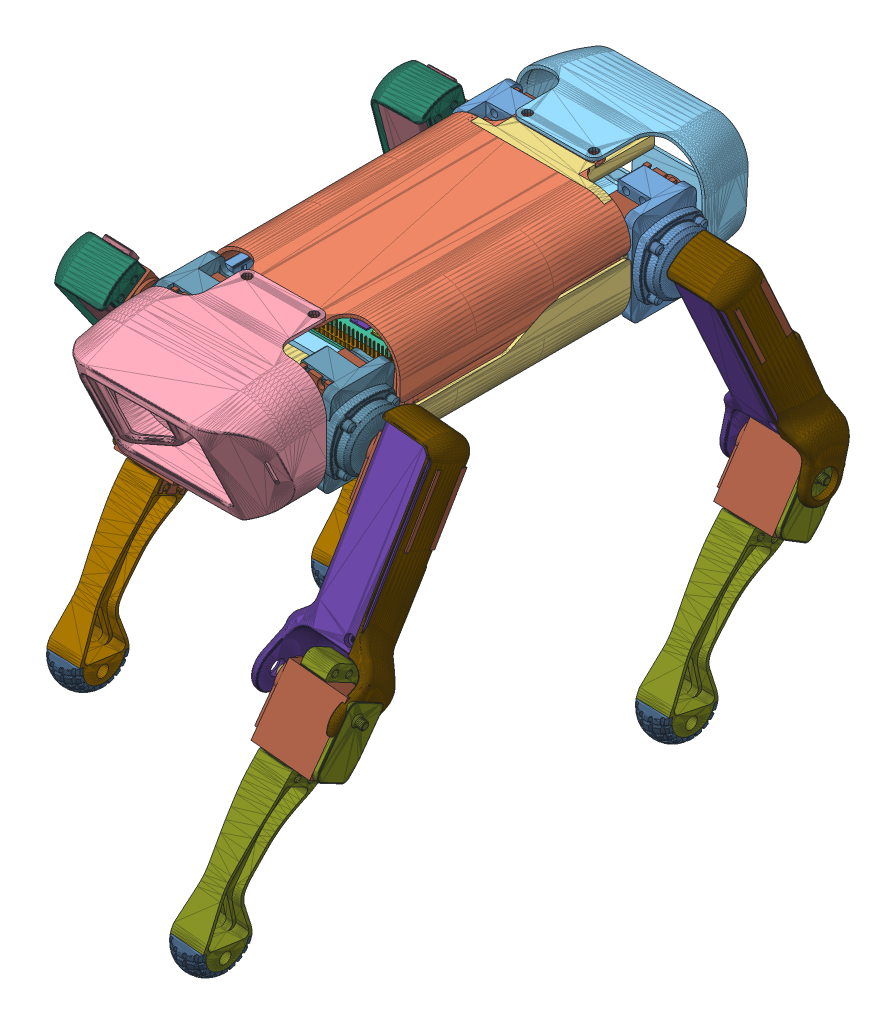
SolidWorks assembly robot_dog, configuration Default. Lengths in mm.
Overall size (261.86 298.31 449.5).
99 component instances, 41 part files, 20 mates.
Components (placement in the parent):
- torsol-1: torsol [Default] at (84.8958 -47.9637 220.9974) size (110 70.14 237.21)
  - R_side_plate_raspberry-1: R_side_plate_raspberry [Default] at (-145.3547 -0.5404 -42.0354) x (1 0 0) z (0 -1 0) size (6.5 130 29)
  - non-mega_L_side_plate-2: non-mega_L_side_plate [Default] at (-41.8547 39.5958 -42.0354) x (-1 0 0) z (0 1 0) size (6.5 130 29)
  - O_shoulder-1: O_shoulder [Default] at (-38.1905 81.6503 -93.0354) x (-1 0 0) z (0 -1 0) size (110 5.21 66) (hidden)
  - I_shoulder_mg-1: I_shoulder_mg [Default] at (-38.6047 81.5958 -42.0354) x (-1 0 0) z (0 -1 0) size (110 51 70)
  - I_shoulder_mg-2: I_shoulder_mg [Default] at (-148.6047 81.4596 87.9646) x (1 0 0) z (0 -1 0) size (110 51 70) (hidden)
  - O_shoulder-2: O_shoulder [Default] at (-148.6047 81.4596 138.9646) x (1 0 0) z (0 -1 0) size (110 5.21 66)
  - plate_with_raspberry-1: plate_with_raspberry [Default] at (-77.9429 -68.9542 72.5105) x (1 0 0) z (0 1 0) size (107 125 22.11)
    - plate_raspberry-1: plate_raspberry [Default] at (-15.1617 3.5459 105.55) size (107 125 2.9)
    - Raspberry Pi 4 Model B-1: Raspberry Pi 4 Model B [Default] at (-14.6617 24.5459 110.6608) x (-1 0 0) z (0 1 0) size (88.99 19.9 58.4)
      - PCB, RPi4ModelB-1: PCB, RPi4ModelB [Default] at origin size (85 1.6 56)
      - Broadcom BCM2711B0 CPU, RPi4ModelB-1: Broadcom BCM2711B0 CPU, RPi4ModelB [Default] at (-13.25 0.8 -4.5) size (15 2.3 15)
      - 2.54 mm DUPONT MALE PIN HEADER, POE, 2X2, RPi4ModelB-1: 2.54 mm DUPONT MALE PIN HEADER, POE, 2X2, RPi4ModelB [Default] at (19 0.8 -18.5) size (5.08 11.3 5.08)
      - 2.54 mm DUPONT MALE PIN HEADER, IO, 2X20, RPi4ModelB-1: 2.54 mm DUPONT MALE PIN HEADER, IO, 2X20, RPi4ModelB [Default] at (-10 0.8 -24.5) size (50.8 11.3 5.08)
      - Camera Connector, RPi4ModelB-1: Camera Connector, RPi4ModelB [Default] at (4 0.8 16.5) x (0 0 -1) z (1 0 0) size (22.4 5.68 5.07)
      - Microphone Plug, RPi4ModelB-1: Microphone Plug, RPi4ModelB [Default] at (11.5 0.8 21.65) size (7.23 7.55 15)
      - Display Connector, RPi4ModelB-1: Display Connector, RPi4ModelB [Default] at (-38.5 0.8 0) x (0 0 1) z (-1 0 0) size (22.4 5.68 5.07)
      - Gigabit Ethernet Port, RPi4ModelB-1: Gigabit Ethernet Port, RPi4ModelB [Default] at (45.5 7.55 -17.75) x (0 0 -1) z (1 0 0) size (16.2 17.24 21.64)
      - Female Micro HDMI Connector, RPi4ModelB-2: Female Micro HDMI Connector, RPi4ModelB [Default] at (-3 0.8 27.3875) size (6.5 3.51 7.5)
      - Female Micro HDMI Connector, RPi4ModelB-3: Female Micro HDMI Connector, RPi4ModelB [Default] at (-16.5 0.8 27.3875) size (6.5 3.51 7.5)
      - Female USB Type C Connector, RPi4ModelB-1: Female USB Type C Connector, RPi4ModelB [Default] at (-31.3 0.8 26.5419) size (8.94 3.96 7.9)
      - 2X USB3.0 PORTS, RPi4ModelB-2: 2X USB3.0 PORTS, RPi4ModelB [Default] at (37.07 0.8 1) size (17.47 19.41 15.68)
      - 91D77 D9WHV 778K, 4 GB LPDDR4 SDRAM, RPi4ModelB-1: 91D77 D9WHV 778K, 4 GB LPDDR4 SDRAM, RPi4ModelB [Default] at (2.25 0.8 -4.5) size (10 0.8 14.5)
      - Cypress CYW43455 Wireless Module Cover, RPi4ModelB-1: Cypress CYW43455 Wireless Module Cover, RPi4ModelB [Default] at (-30.5 0.8 -14.5) size (11 1.6 13)
      - SD Card Slot, RPi4ModelB-1: SD Card Slot, RPi4ModelB [Default] at (-35.3 -0.8 0) x (0 0 -1) z (-1 0 0) size (11.95 1.45 11.4)
      - VIA VL805 PCIe USB 3.0 controller, RPi4ModelB-1: VIA VL805 PCIe USB 3.0 controller, RPi4ModelB [Default] at (17.5 0.8 4) size (8.8 0.8 8.8)
      - 2X USB2.0 PORTS, RPi4ModelB-1: 2X USB2.0 PORTS, RPi4ModelB [Default] at (37.065 0.65 19) size (17.87 19.16 15.33)
      - Broadcom BCM54213PE Gigabit Ethernet Transceiver, RPi4ModelB-1: Broadcom BCM54213PE Gigabit Ethernet Transceiver, RPi4ModelB [Default] at (16.5 0.8 -10) size (6.8 1 6.8)
      - MxL7704 Universal PMIC, RPi4ModelB-1: MxL7704 Universal PMIC, RPi4ModelB [Default] at (-32.5 0.8 16) size (5.4 0.8 5.4)
  - copper_cylinder-1: copper_cylinder [Default] at (-111.6047 62.4966 72.4646) x (-0.975868 0 -0.218361) z (0 -1 0) size (3 3 20)
  - copper_cylinder-2: copper_cylinder [Default] at (-53.6047 62.4966 72.4646) x (-0.932816 0 0.360352) z (0 -1 0) size (3 3 20)
  - copper_cylinder-3: copper_cylinder [Default] at (-53.6047 62.4966 23.4646) x (-0.581089 0 -0.81384) z (0 -1 0) size (3 3 20)
  - copper_cylinder-4: copper_cylinder [Default] at (-111.6047 62.4966 23.4646) x (-0.873325 0 -0.487138) z (0 -1 0) size (3 3 20)
  - plate_top_raspberry-1: plate_top_raspberry [Default] at (-93.1414 65.3966 64.4169) x (1 0 0) z (0 -1 0) size (85.07 56 2.9)
  - battery_4000mah_2s-1: battery_4000mah_2s [Default] at (-135.6047 66.4958 13.9646) x (1 0 0) z (0 -1 0) size (85 42 27)
- right_foot_front-1: right_foot_front [Default] at (-126.7235 -93.0726 453.4039) x (-0.034309 -0.880659 0.472507) z (-0.018394 -0.472149 -0.881327) size (236.52 96.4 141.61) (flexible)
  - R_wrist_mg-1: R_wrist_mg [Default] at (-88.5645 -25.7472 139.9903) size (149.99 36.9 30)
  - foot-1: foot [Default] at (37.4355 -5.9472 149.9903) x (0.342021 0 -0.939692) z (-0.939692 0 -0.342021) size (38.32 20 19.41)
  - MG996R-1: MG996R [Default] at (-68.3145 3.2528 149.9903) x (1 0 0) z (0 0 -1) size (54.5 43 20)
    - servo-1: servo [Default] at origin size (54.5 39 20)
    - shaft-1: shaft [Default] at (-10.1089 43 0) x (-0.837169 0 -0.546944) z (-0.546944 0 0.837169) size (5.9 19.57 5.9)
  - R_arm_mg-1: R_arm_mg [Default] at (-134.0023 -85.7472 46.9151) x (-0.895965 0 0.444124) z (0.444124 0 0.895965) size (38.24 39.8 137.4)
  - MG996R-2: MG996R [Default] at (-133.9685 -3.7472 69.4996) x (0.444124 0 0.895965) z (0.895965 0 -0.444124) size (54.5 43 20)
    - servo-1: servo [Default] at origin size (54.5 39 20)
    - shaft-1: shaft [Default] at (-10.1089 43 0) x (-0.837169 0 -0.546944) z (-0.546944 0 0.837169) size (5.9 19.57 5.9)
  - R_arm_joint_mg-1: R_arm_joint_mg [Default] at (-161.1481 -115.2472 59.9077) x (0 -1 0) z (0.881327 0 0.472507) size (37.5 46 56.5)
  - R_arm_cover-1: R_arm_cover [Default] at (-129.9927 -48.0472 37.1147) x (-0.895965 0 0.444124) z (0.444124 0 0.895965) size (41.16 45 143.55)
  - MG996R-3: MG996R [Default] at (-146.1363 -75.2472 74.7639) x (0.881327 0 0.472507) z (0 1 0) size (54.5 43 20)
    - servo-1: servo [Default] at origin size (54.5 39 20)
    - shaft-1: shaft [Default] at (-10.1089 43 0) x (-0.837169 0 -0.546944) z (-0.546944 0 0.837169) size (5.9 19.57 5.9)
- left_foot_back-1: left_foot_back [Default] at (93.3781 -108.8977 296.0109) x (-0.021318 -0.848929 0.528077) z (-0.013257 -0.527911 -0.849196) size (284.28 93.4 85.82) (flexible)
  - L_wrist_mg-1: L_wrist_mg [Default] at (-104.9134 49.2874 139.9903) size (149.99 36.9 30)
  - foot-1: foot [Default] at (21.0866 19.2874 149.9903) x (0.342019 0 -0.939693) z (-0.939693 0 -0.342019) size (38.32 20 19.41)
  - MG996R-1: MG996R [Default] at (-84.6634 -9.7126 149.9903) size (54.5 43 20)
    - servo-1: servo [Default] at origin size (54.5 39 20)
    - shaft-1: shaft [Default] at (-10.1089 43 0) x (-0.837169 0 -0.546944) z (-0.546944 0 0.837169) size (5.9 19.57 5.9)
  - L_arm_mg-1: L_arm_mg [Default] at (-161.6203 26.2874 53.9721) x (-0.838875 0 0.544324) z (0.544324 0 0.838875) size (38.24 39.8 137.4)
  - MG996R-2: MG996R [Default] at (-158.9865 -5.7126 76.4026) x (0.544324 0 0.838875) z (-0.838875 0 0.544324) size (54.5 43 20)
    - servo-1: servo [Default] at origin size (54.5 39 20)
    - shaft-1: shaft [Default] at (-10.1089 43 0) x (-0.837169 0 -0.546944) z (-0.546944 0 0.837169) size (5.9 19.57 5.9)
  - L_arm_cover-1: L_arm_cover [Default] at (-160.8168 28.5874 45.1062) x (-0.838875 0 0.544324) z (0.544324 0 0.838875) size (41.16 45 143.55)
  - L_arm_joint_mg-1: L_arm_joint_mg [Default] at (-141.9481 74.7874 69.9359) x (0 -1 0) z (-0.849196 0 -0.528077) size (37.5 46 56.5)
  - MG996R-3: MG996R [Default] at (-156.825 65.7874 53.6191) x (0.849196 0 0.528077) z (0 -1 0) size (54.5 43 20)
    - servo-1: servo [Default] at origin size (54.5 39 20)
    - shaft-1: shaft [Default] at (-10.1089 43 0) x (-0.837169 0 -0.546944) z (-0.546944 0 0.837169) size (5.9 19.57 5.9)
- left_foot_front-1: left_foot_front [Default] at (86.019 -111.7023 568.2939) x (-0.086144 -0.870613 0.484368) z (-0.047693 -0.482014 -0.874864) size (271.86 94.6 110.14) (flexible)
  - L_wrist_mg-1: L_wrist_mg [Default] at (-104.9134 49.2874 139.9903) size (149.99 36.9 30)
  - foot-1: foot [Default] at (21.0866 19.2874 149.9903) x (0.342019 0 -0.939693) z (-0.939693 0 -0.342019) size (38.32 20 19.41)
  - MG996R-1: MG996R [Default] at (-84.6634 -9.7126 149.9903) size (54.5 43 20)
    - servo-1: servo [Default] at origin size (54.5 39 20)
    - shaft-1: shaft [Default] at (-10.1089 43 0) x (-0.837169 0 -0.546944) z (-0.546944 0 0.837169) size (5.9 19.57 5.9)
  - L_arm_mg-1: L_arm_mg [Default] at (-211.4877 30.2874 141.8872) x (-0.101729 0 0.994812) z (0.994812 0 0.101729) size (38.24 39.8 137.4)
  - MG996R-2: MG996R [Default] at (-192.3601 -1.7126 153.8953) x (0.994812 0 0.101729) z (-0.101729 0 0.994812) size (54.5 43 20)
    - servo-1: servo [Default] at origin size (54.5 39 20)
    - shaft-1: shaft [Default] at (-10.1089 43 0) x (-0.837169 0 -0.546944) z (-0.546944 0 0.837169) size (5.9 19.57 5.9)
  - L_arm_cover-1: L_arm_cover [Default] at (-217.8919 32.5874 135.7036) x (-0.101729 0 0.994812) z (0.994812 0 0.101729) size (41.16 45 143.55)
  - MG996R-3: MG996R [Default] at (-210.2875 66.9874 167.0835) x (0.874864 0 0.484368) z (0 1 0) size (54.5 43 20)
    - servo-1: servo [Default] at origin size (54.5 39 20)
    - shaft-1: shaft [Default] at (-10.1089 43 0) x (-0.837169 0 -0.546944) z (-0.546944 0 0.837169) size (5.9 19.57 5.9)
  - R_arm_joint_mg-1: R_arm_joint_mg [Default] at (-189.6653 106.9874 171.6427) x (0 1 0) z (-0.874864 0 -0.484368) size (37.5 46 56.5)
- right_foot_back-1: right_foot_back [Default] at (-115.1028 -105.3329 309.254) x (0.02206 -0.868899 0.494498) z (0.012551 -0.494339 -0.869179) size (200.98 91.6 160.78) (flexible)
  - R_wrist_mg-1: R_wrist_mg [Default] at (-88.5645 -25.7472 139.9903) size (149.99 36.9 30)
  - foot-1: foot [Default] at (37.4355 -5.9472 149.9903) x (0.342021 0 -0.939692) z (-0.939692 0 -0.342021) size (38.32 20 19.41)
  - MG996R-1: MG996R [Default] at (-68.3145 3.2528 149.9903) x (1 0 0) z (0 0 -1) size (54.5 43 20)
    - servo-1: servo [Default] at origin size (54.5 39 20)
    - shaft-1: shaft [Default] at (-10.1089 43 0) x (-0.837169 0 -0.546944) z (-0.546944 0 0.837169) size (5.9 19.57 5.9)
  - R_arm_mg-1: R_arm_mg [Default] at (-166.5461 -85.7472 72.8675) x (-0.684015 0 0.729468) z (0.729468 0 0.684015) size (38.24 39.8 137.4)
  - MG996R-2: MG996R [Default] at (-158.6145 -3.7472 94.0135) x (0.729468 0 0.684015) z (0.684015 0 -0.729468) size (54.5 43 20)
    - servo-1: servo [Default] at origin size (54.5 39 20)
    - shaft-1: shaft [Default] at (-10.1089 43 0) x (-0.837169 0 -0.546944) z (-0.546944 0 0.837169) size (5.9 19.57 5.9)
  - R_arm_cover-1: R_arm_cover [Default] at (-166.2178 -48.0472 62.2838) x (-0.684015 0 0.729468) z (0.729468 0 0.684015) size (41.16 45 143.55)
  - MG996R-3: MG996R [Default] at (-157.9418 -70.4472 73.046) x (0.869179 0 0.494498) z (0 -1 0) size (54.5 43 20)
    - servo-1: servo [Default] at origin size (54.5 39 20)
    - shaft-1: shaft [Default] at (-10.1089 43 0) x (-0.837169 0 -0.546944) z (-0.546944 0 0.837169) size (5.9 19.57 5.9)
  - L_arm_joint_mg-1: L_arm_joint_mg [Default] at (-178.5097 -80.4472 68.2475) x (0 1 0) z (0.869179 0 0.494498) size (37.5 46 56.5)
- non-mega_T_cover_mg-1: non-mega_T_cover_mg [Default] at (-65.4072 -90.53 364.1871) x (-0.004263 0.000801 -0.999991) z (0.999991 0 -0.004263) size (180 34.5 114)
- non-mega_B_cover_mg-1: non-mega_B_cover_mg [Default] at (-65.8721 -36.5293 363.9553) x (0 0.000778 -1) z (1 0 0) size (180 42.5 114)
- F_cover-1: F_cover [Default] at (48.4963 35.3945 333.4551) x (0.008769 -0.000778 0.999961) z (0 -1 -0.000778) size (92.81 114 70)
- R_cover-1: R_cover [Default] at (-66.43 33.5613 124.2887) x (-0.000003 -1 -0.000778) z (0.004263 -0.000778 0.999991) size (70 114 69.85)
Mates (geometry in assembly coordinates):
- Parallel2: parallel aligned: plane of torsol-1/O_shoulder-2 through (-63.7089 33.4959 362.262) normal (0 0 1); plane of right_foot_front-1/MG996R-3/shaft-1 through (-47.5013 7.4959 361.462) normal (0 0 1)
- Coincident9: coincident anti-aligned: line of torsol-1/O_shoulder-2 through (-47.5013 7.4959 362.262) axis (0 0 1); line of right_foot_front-1/MG996R-3/shaft-1 through (-47.5013 7.4959 361.462) axis (0 0 -1)
- Coincident10: coincident anti-aligned: plane of torsol-1/I_shoulder_mg-2 through (-63.7089 33.4959 313.962) normal (0 0 1); plane of right_foot_front-1/R_arm_joint_mg-1 through (-7.1368 16.0722 313.962) normal (0 0 -1)
- Coincident12: coincident anti-aligned: line of torsol-1/O_shoulder-1 through (30.4976 7.6867 125.662) axis (0 0 -1); line of left_foot_back-1/MG996R-3/shaft-1 through (30.4976 7.6867 124.662) axis (0 0 1)
- Distance3: distance = 1 mm aligned: plane of left_foot-1/MG996R-3/shaft-1 through (30.4976 7.6867 124.662) normal (0 0 -1); plane of torsol-1/O_shoulder-1 through (46.7052 33.6867 125.662) normal (0 0 -1)
- Coincident13: coincident anti-aligned: line of torsol-1/O_shoulder-2 through (30.4987 7.4959 362.262) axis (0 0 1); line of left_foot_front-1/MG996R-3/shaft-1 through (30.4987 7.4959 363.262) axis (0 0 -1)
- Distance4: distance = 1 mm aligned: plane of left_foot_front-1/MG996R-3/shaft-1 through (30.4987 7.4959 363.262) normal (0 0 1); plane of torsol-1/O_shoulder-2 through (-63.7089 33.4959 362.262) normal (0 0 1)
- Coincident15: coincident anti-aligned: line of torsol-1/O_shoulder-1 through (-47.5024 7.6867 125.662) axis (0 0 -1); line of right_foot_back-1/MG996R-3/shaft-1 through (-47.5024 7.6867 124.662) axis (0 0 1)
- Distance5: distance = 1 mm aligned: plane of right_foot_back-1/MG996R-3/shaft-1 through (-47.5024 7.6867 124.662) normal (0 0 -1); plane of torsol-1/O_shoulder-1 through (46.7052 33.6867 125.662) normal (0 0 -1)
- Coincident19: coincident: point of torsol-1/I_shoulder_mg-2; point of non-mega_T_cover_mg-1
- Coincident20: coincident: line of torsol-1/I_shoulder_mg-2 through (-29.1961 31.4959 331.516) axis (-0.951057 0 -0.309017); point of non-mega_T_cover_mg-1
- Coincident22: coincident: plane of torsol-1/I_shoulder_mg-1 through (46.2911 31.6321 178.962) normal (0 1 0); point of non-mega_T_cover_mg-1
- Coincident23: coincident: point of torsol-1/I_shoulder_mg-2; point of non-mega_B_cover_mg-1
- Coincident24: coincident: line of torsol-1/I_shoulder_mg-2 through (-3.2217 -34.5041 331.516) axis (-0.998027 0 0.06279); point of non-mega_B_cover_mg-1
- Coincident25: coincident: plane of torsol-1/I_shoulder_mg-1 through (46.2911 -34.3679 178.962) normal (0 -1 0); point of non-mega_B_cover_mg-1
- Coincident26: coincident: point of non-mega_T_cover_mg-1; point of F_cover-1
- Coincident27: coincident: line of non-mega_T_cover_mg-1 through (12.1055 33.5 326.4443) axis (-0.991992 0.000105 -0.126301); point of F_cover-1
- Parallel5: parallel anti-aligned: plane of non-mega_B_cover_mg-1 through (-65.8721 -36.5293 363.9553) normal (0 -1 -0.000778); plane of F_cover-1 through (48.4963 -32.7055 333.4021) normal (0 1 0.000778)
- Coincident31: coincident: point of non-mega_T_cover_mg-1; point of R_cover-1
- Coincident32: coincident: line of non-mega_T_cover_mg-1 through (-29.9433 33.6321 161.6449) axis (0.991993 -0.000105 0.12629); point of R_cover-1
